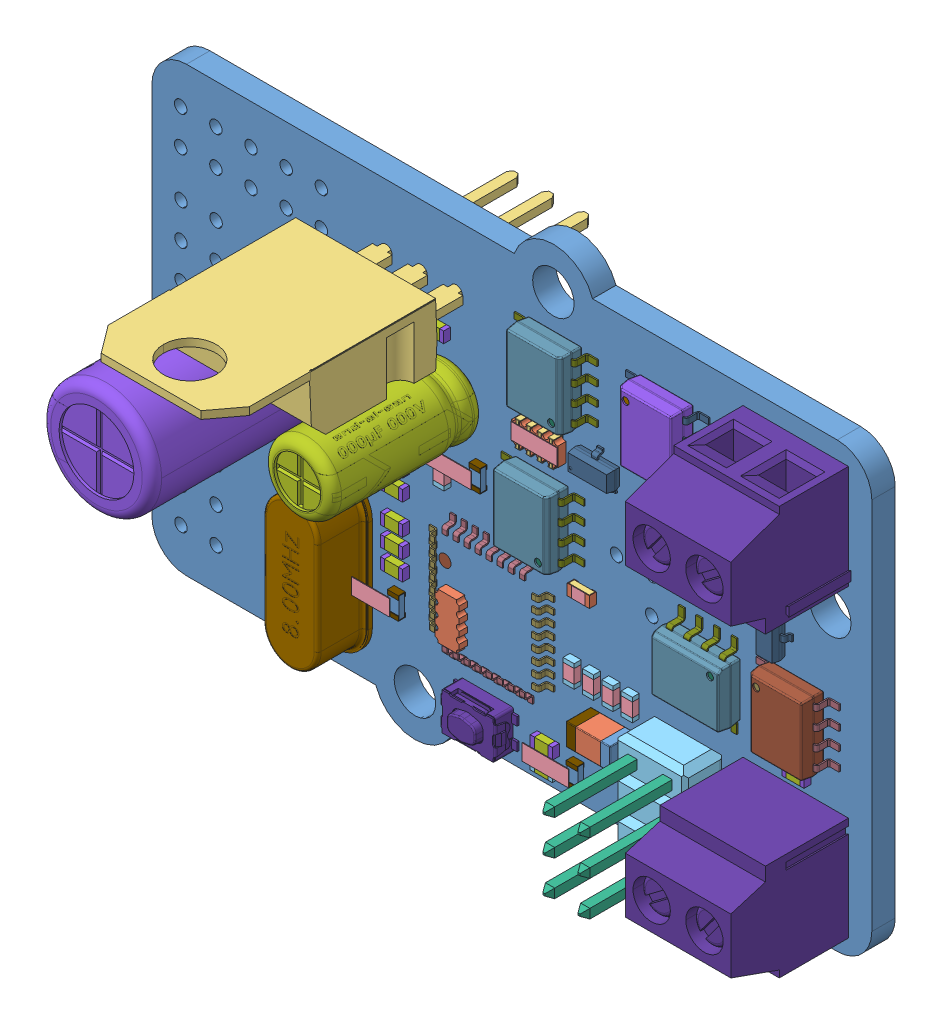
SolidWorks assembly DMotor_Rev1, configuration По умолчанию. Lengths in mm.
Overall size (52 36 28.9).
344 component instances, 44 part files, 0 mates.
Components (placement in the parent):
- DMotor_Rev1.step-1: DMotor_Rev1.step [По умолчанию] at origin size (52 36 28.9)
  - Board.step-1: Board.step [По умолчанию] at origin size (52 36 1.69)
    - Open CASCADE STEP translator 6.8 1.1.1.step-1: Open CASCADE STEP translator 6.8 1.1.1.step [По умолчанию] at (0 0 -1.692) size (52 36 1.69)
  - RN1.step-1: RN1.step [По умолчанию] at origin size (3.35 1.85 0.7)
    - 5778449216.step-1: 5778449216.step [По умолчанию] at (28.3 21.5 0) x (0 1 0) z (0 0 1) size (1.85 3.35 0.7)
      - body.step-1: body.step [По умолчанию] at (-0.875 -1.675 0) size (1.75 3.35 0.6)
        - Open_CASCADE_STEP_translator_6.8_25.1.1.step-1: Open_CASCADE_STEP_translator_6.8_25.1.1.step [По умолчанию] at origin size (1.75 3.35 0.6)
      - Mid_Pin.step-1: Mid_Pin.step [По умолчанию] at (-0.875 -1.2 0) size (0.3 0.38 0.7)
        - Open_CASCADE_STEP_translator_6.8_25.3.1.step-1: Open_CASCADE_STEP_translator_6.8_25.3.1.step [По умолчанию] at origin size (0.3 0.38 0.7)
      - Mid_Pin.step-2: Mid_Pin.step [По умолчанию] at (0.875 1.2 0) x (-1 0 0) z (0 0 1) size (0.3 0.38 0.7)
        - Open_CASCADE_STEP_translator_6.8_25.3.1.step-1: Open_CASCADE_STEP_translator_6.8_25.3.1.step [По умолчанию] at origin size (0.3 0.38 0.7)
      - Mid_Pin.step-3: Mid_Pin.step [По умолчанию] at (-0.875 -0.4 0) size (0.3 0.38 0.7)
        - Open_CASCADE_STEP_translator_6.8_25.3.1.step-1: Open_CASCADE_STEP_translator_6.8_25.3.1.step [По умолчанию] at origin size (0.3 0.38 0.7)
      - Mid_Pin.step-4: Mid_Pin.step [По умолчанию] at (0.875 0.4 0) x (-1 0 0) z (0 0 1) size (0.3 0.38 0.7)
        - Open_CASCADE_STEP_translator_6.8_25.3.1.step-1: Open_CASCADE_STEP_translator_6.8_25.3.1.step [По умолчанию] at origin size (0.3 0.38 0.7)
      - Mid_Pin.step-5: Mid_Pin.step [По умолчанию] at (-0.875 0.4 0) size (0.3 0.38 0.7)
        - Open_CASCADE_STEP_translator_6.8_25.3.1.step-1: Open_CASCADE_STEP_translator_6.8_25.3.1.step [По умолчанию] at origin size (0.3 0.38 0.7)
      - Mid_Pin.step-6: Mid_Pin.step [По умолчанию] at (0.875 -0.4 0) x (-1 0 0) z (0 0 1) size (0.3 0.38 0.7)
        - Open_CASCADE_STEP_translator_6.8_25.3.1.step-1: Open_CASCADE_STEP_translator_6.8_25.3.1.step [По умолчанию] at origin size (0.3 0.38 0.7)
      - Mid_Pin.step-7: Mid_Pin.step [По умолчанию] at (-0.875 1.2 0) size (0.3 0.38 0.7)
        - Open_CASCADE_STEP_translator_6.8_25.3.1.step-1: Open_CASCADE_STEP_translator_6.8_25.3.1.step [По умолчанию] at origin size (0.3 0.38 0.7)
      - Mid_Pin.step-8: Mid_Pin.step [По умолчанию] at (0.875 -1.2 0) x (-1 0 0) z (0 0 1) size (0.3 0.38 0.7)
        - Open_CASCADE_STEP_translator_6.8_25.3.1.step-1: Open_CASCADE_STEP_translator_6.8_25.3.1.step [По умолчанию] at origin size (0.3 0.38 0.7)
      - mark.step-1: mark.step [По умолчанию] at (-0.875 -1.675 0) size (1.15 3.35 0.05)
  - ICSP.step-1: ICSP.step [По умолчанию] at origin size (5.08 7.62 12.7)
    - 2x3_TH_Pitch_2_54mm.step-1: 2x3_TH_Pitch_2_54mm.step [По умолчанию] at (38.7601 0.89 0) x (0 1 0) z (1 0 0) size (7.62 12.7 5.08)
      - header2x3.step-1: header2x3.step [По умолчанию] at (0 1.4 0) size (7.62 2.8 5.08)
      - pin.step-1: pin.step [По умолчанию] at (1.29 -3.5 1.29) size (0.67 12.7 0.67)
      - pin.step-2: pin.step [По умолчанию] at (1.29 -3.5 -1.25) size (0.67 12.7 0.67)
      - pin.step-3: pin.step [По умолчанию] at (3.83 -3.5 1.29) size (0.67 12.7 0.67)
      - pin.step-4: pin.step [По умолчанию] at (3.83 -3.5 -1.25) size (0.67 12.7 0.67)
      - pin.step-5: pin.step [По умолчанию] at (6.37 -3.5 1.29) size (0.67 12.7 0.67)
      - pin.step-6: pin.step [По умолчанию] at (6.37 -3.5 -1.25) size (0.67 12.7 0.67)
  - C9.step-1: C9.step [По умолчанию] at origin size (1.6 0.8 0.5)
    - 5928350752.step-1: 5928350752.step [По умолчанию] at (17.8 11.1 0) size (1 0.8 0.5)
      - Extruded.step-1: Extruded.step [По умолчанию] at origin size (1 0.8 0.5)
    - 5928351312.step-1: 5928351312.step [По умолчанию] at (18.45 11.1 0) size (0.3 0.8 0.5)
      - Extruded-0.step-1: Extruded-0.step [По умолчанию] at origin size (0.3 0.8 0.5)
    - 5928351312.step-2: 5928351312.step [По умолчанию] at (17.15 11.1 0) size (0.3 0.8 0.5)
      - Extruded-0.step-1: Extruded-0.step [По умолчанию] at origin size (0.3 0.8 0.5)
  - C11.step-1: C11.step [По умолчанию] at origin size (1.6 0.8 0.5)
    - 5928350752.step-1: 5928350752.step [По умолчанию] at (17.8 8.3 0) size (1 0.8 0.5)
      - Extruded.step-1: Extruded.step [По умолчанию] at origin size (1 0.8 0.5)
    - 5928351312.step-1: 5928351312.step [По умолчанию] at (18.45 8.3 0) size (0.3 0.8 0.5)
      - Extruded-0.step-1: Extruded-0.step [По умолчанию] at origin size (0.3 0.8 0.5)
    - 5928351312.step-2: 5928351312.step [По умолчанию] at (17.15 8.3 0) size (0.3 0.8 0.5)
      - Extruded-0.step-1: Extruded-0.step [По умолчанию] at origin size (0.3 0.8 0.5)
  - Y1.step-1: Y1.step [По умолчанию] at origin size (4.65 11.35 5.59)
    - HC-49S.step-1: HC-49S.step [По умолчанию] at (13.6 6.8251 0) x (0 1 0) z (1 0 0) size (11.35 5.59 4.65)
  - VT2.step-1: VT2.step [По умолчанию] at origin size (2.9 2.3 1)
    - SOT23-3.step-1: SOT23-3.step [По умолчанию] at (31 21.9 0) x (1 0 0) z (0 -1 0) size (2.9 1 2.3)
  - VT1.step-1: VT1.step [По умолчанию] at origin size (2.3 2.9 1)
    - SOT23-3.step-1: SOT23-3.step [По умолчанию] at (45.2 19.5 0) x (0 -1 0) z (-1 0 0) size (2.9 1 2.3)
  - U1.step-1: U1.step [По умолчанию] at origin size (9 9 1.11)
    - 5778452896.step-1: 5778452896.step [По умолчанию] at (24.6 9.05 0) size (9 9 1.11)
      - body.step-1: body.step [По умолчанию] at (-3.5 -3.5 0) size (1.75 3.35 0.6)
        - Open_CASCADE_STEP_translator_6.8_25.1.1.step-1: Open_CASCADE_STEP_translator_6.8_25.1.1.step [По умолчанию] at origin size (1.75 3.35 0.6)
      - Open_CASCADE_STEP_translator_6.8_22.1.step-1: Open_CASCADE_STEP_translator_6.8_22.1.step [По умолчанию] at (-3.5 -3.5 0.001) size (0.89 0.89 0.01)
      - Leader.step-1: Leader.step [По умолчанию] at (-3.5 -2.8 0) x (-1 0 0) z (0 0 1) size (1 0.38 0.68)
      - Leader.step-2: Leader.step [По умолчанию] at (-3.5 -2 0) x (-1 0 0) z (0 0 1) size (1 0.38 0.68)
      - Leader.step-3: Leader.step [По умолчанию] at (-3.5 -1.2 0) x (-1 0 0) z (0 0 1) size (1 0.38 0.68)
      - Leader.step-4: Leader.step [По умолчанию] at (-3.5 -0.4 0) x (-1 0 0) z (0 0 1) size (1 0.38 0.68)
      - Leader.step-5: Leader.step [По умолчанию] at (-3.5 0.4 0) x (-1 0 0) z (0 0 1) size (1 0.38 0.68)
      - Leader.step-6: Leader.step [По умолчанию] at (-3.5 1.2 0) x (-1 0 0) z (0 0 1) size (1 0.38 0.68)
      - Leader.step-7: Leader.step [По умолчанию] at (-3.5 2 0) x (-1 0 0) z (0 0 1) size (1 0.38 0.68)
      - Leader.step-8: Leader.step [По умолчанию] at (-3.5 2.8 0) x (-1 0 0) z (0 0 1) size (1 0.38 0.68)
      - Leader.step-9: Leader.step [По умолчанию] at (3.5 -2.8 0) size (1 0.38 0.68)
      - Leader.step-10: Leader.step [По умолчанию] at (3.5 -2 0) size (1 0.38 0.68)
      - Leader.step-11: Leader.step [По умолчанию] at (3.5 -1.2 0) size (1 0.38 0.68)
      - Leader.step-12: Leader.step [По умолчанию] at (3.5 -0.4 0) size (1 0.38 0.68)
      - Leader.step-13: Leader.step [По умолчанию] at (3.5 0.4 0) size (1 0.38 0.68)
      - Leader.step-14: Leader.step [По умолчанию] at (3.5 1.2 0) size (1 0.38 0.68)
      - Leader.step-15: Leader.step [По умолчанию] at (3.5 2 0) size (1 0.38 0.68)
      - Leader.step-16: Leader.step [По умолчанию] at (3.5 2.8 0) size (1 0.38 0.68)
      - Leader-1.step-1: Leader-1.step [По умолчанию] at (-2.8 -3.5 0) x (0 -1 0) z (0 0 1) size (1 0.38 0.68)
      - Leader-1.step-2: Leader-1.step [По умолчанию] at (-2 -3.5 0) x (0 -1 0) z (0 0 1) size (1 0.38 0.68)
      - Leader-1.step-3: Leader-1.step [По умолчанию] at (-1.2 -3.5 0) x (0 -1 0) z (0 0 1) size (1 0.38 0.68)
      - Leader-1.step-4: Leader-1.step [По умолчанию] at (-0.4 -3.5 0) x (0 -1 0) z (0 0 1) size (1 0.38 0.68)
      - Leader-1.step-5: Leader-1.step [По умолчанию] at (0.4 -3.5 0) x (0 -1 0) z (0 0 1) size (1 0.38 0.68)
      - Leader-1.step-6: Leader-1.step [По умолчанию] at (1.2 -3.5 0) x (0 -1 0) z (0 0 1) size (1 0.38 0.68)
      - Leader-1.step-7: Leader-1.step [По умолчанию] at (2 -3.5 0) x (0 -1 0) z (0 0 1) size (1 0.38 0.68)
      - Leader-1.step-8: Leader-1.step [По умолчанию] at (2.8 -3.5 0) x (0 -1 0) z (0 0 1) size (1 0.38 0.68)
      - Leader-1.step-9: Leader-1.step [По умолчанию] at (-2.8 3.5 0) x (0 1 0) z (0 0 1) size (1 0.38 0.68)
      - Leader-1.step-10: Leader-1.step [По умолчанию] at (-2 3.5 0) x (0 1 0) z (0 0 1) size (1 0.38 0.68)
      - Leader-1.step-11: Leader-1.step [По умолчанию] at (-1.2 3.5 0) x (0 1 0) z (0 0 1) size (1 0.38 0.68)
      - Leader-1.step-12: Leader-1.step [По умолчанию] at (-0.4 3.5 0) x (0 1 0) z (0 0 1) size (1 0.38 0.68)
      - Leader-1.step-13: Leader-1.step [По умолчанию] at (0.4 3.5 0) x (0 1 0) z (0 0 1) size (1 0.38 0.68)
      - Leader-1.step-14: Leader-1.step [По умолчанию] at (1.2 3.5 0) x (0 1 0) z (0 0 1) size (1 0.38 0.68)
      - Leader-1.step-15: Leader-1.step [По умолчанию] at (2 3.5 0) x (0 1 0) z (0 0 1) size (1 0.38 0.68)
      - Leader-1.step-16: Leader-1.step [По умолчанию] at (2.8 3.5 0) x (0 1 0) z (0 0 1) size (1 0.38 0.68)
  - U2.step-1: U2.step [По умолчанию] at origin size (6 5.01 1.75)
    - 5778448736.step-1: 5778448736.step [По умолчанию] at (28.3 17.1 0) x (-1 0 0) z (0 0 1) size (6 5 1.75)
      - Body-1.step-1: Body-1.step [По умолчанию] at (-2 -2.5 0) size (4 5 1.65)
        - Open_CASCADE_STEP_translator_6.8_4.2.1.step-1: Open_CASCADE_STEP_translator_6.8_4.2.1.step [По умолчанию] at origin size (4 5 1.65)
      - Open_CASCADE_STEP_translator_6.8_4.1.step-1: Open_CASCADE_STEP_translator_6.8_4.1.step [По умолчанию] at (-2 -2.5 0.001) size (0.51 0.51 0.01)
      - Leader-2.step-1: Leader-2.step [По умолчанию] at (-2 -1.905 0) x (-1 0 0) z (0 0 1) size (1 0.42 0.97)
      - Leader-2.step-2: Leader-2.step [По умолчанию] at (-2 -0.635 0) x (-1 0 0) z (0 0 1) size (1 0.42 0.97)
      - Leader-2.step-3: Leader-2.step [По умолчанию] at (-2 0.635 0) x (-1 0 0) z (0 0 1) size (1 0.42 0.97)
      - Leader-2.step-4: Leader-2.step [По умолчанию] at (-2 1.905 0) x (-1 0 0) z (0 0 1) size (1 0.42 0.97)
      - Leader-2.step-5: Leader-2.step [По умолчанию] at (2 -1.905 0) size (1 0.42 0.97)
      - Leader-2.step-6: Leader-2.step [По умолчанию] at (2 -0.635 0) size (1 0.42 0.97)
      - Leader-2.step-7: Leader-2.step [По умолчанию] at (2 0.635 0) size (1 0.42 0.97)
      - Leader-2.step-8: Leader-2.step [По умолчанию] at (2 1.905 0) size (1 0.42 0.97)
  - RESET.step-1: RESET.step [По умолчанию] at origin size (4.6 2.8 1.94)
    - KMR221GLFS.step-1: KMR221GLFS.step [По умолчанию] at (24.2249 2.1749 0) x (-1 0 0) z (0 1 0) size (4.6 1.94 2.8)
  - R7.step-1: R7.step [По умолчанию] at origin size (3.35 1.75 1.15)
    - 5778454576.step-1: 5778454576.step [По умолчанию] at (23.8 17 0) x (0 1 0) z (0 0 1) size (1.75 3.35 1.15)
      - Terminal.step-1: Terminal.step [По умолчанию] at (-0.8 -0.4 0) size (0.3 0.8 0.5)
        - Open_CASCADE_STEP_translator_6.8_7.2.1.step-1: Open_CASCADE_STEP_translator_6.8_7.2.1.step [По умолчанию] at origin size (0.3 0.8 0.5)
      - Terminal.step-2: Terminal.step [По умолчанию] at (0.8 0.4 0) x (-1 0 0) z (0 0 1) size (0.3 0.8 0.5)
        - Open_CASCADE_STEP_translator_6.8_7.2.1.step-1: Open_CASCADE_STEP_translator_6.8_7.2.1.step [По умолчанию] at origin size (0.3 0.8 0.5)
      - Mid_Body.step-1: Mid_Body.step [По умолчанию] at (-0.8 -0.4 0) size (1.5 0.8 0.4)
      - mark.step-1: mark.step [По умолчанию] at (-0.5 -0.4 0.45) size (1.15 3.35 0.05)
  - R6.step-1: R6.step [По умолчанию] at origin size (1.6 0.8 0.5)
    - 5778452416.step-1: 5778452416.step [По умолчанию] at (31.3 13.4 0) x (1 0 0) z (0 0 1) size (1.6 0.8 0.5)
      - Terminal-1.step-1: Terminal-1.step [По умолчанию] at (-0.8 -0.4 0) size (0.3 0.8 0.5)
        - Open_CASCADE_STEP_translator_6.8_7.2.1-3.step-1: Open_CASCADE_STEP_translator_6.8_7.2.1-3.step [По умолчанию] at origin size (0.3 0.8 0.5)
      - Terminal-1.step-2: Terminal-1.step [По умолчанию] at (0.8 0.4 0) x (-1 0 0) z (0 0 1) size (0.3 0.8 0.5)
        - Open_CASCADE_STEP_translator_6.8_7.2.1-3.step-1: Open_CASCADE_STEP_translator_6.8_7.2.1-3.step [По умолчанию] at origin size (0.3 0.8 0.5)
      - Mid_Body-4.step-1: Mid_Body-4.step [По умолчанию] at (-0.8 -0.4 0) size (1.5 0.8 0.4)
      - Mark-5.step-1: Mark-5.step [По умолчанию] at (-0.5 -0.4 0.45) size (1 0.8 0.05)
  - R5.step-1: R5.step [По умолчанию] at origin size (1.6 0.8 0.5)
    - 5778448016.step-1: 5778448016.step [По умолчанию] at (28.625 1.175 0) x (-1 0 0) z (0 0 1) size (1.6 0.8 0.5)
      - Terminal-2.step-1: Terminal-2.step [По умолчанию] at (-0.8 -0.4 0) size (0.3 0.8 0.5)
        - Open_CASCADE_STEP_translator_6.8_7.2.1-6.step-1: Open_CASCADE_STEP_translator_6.8_7.2.1-6.step [По умолчанию] at origin size (0.3 0.8 0.5)
      - Terminal-2.step-2: Terminal-2.step [По умолчанию] at (0.8 0.4 0) x (-1 0 0) z (0 0 1) size (0.3 0.8 0.5)
        - Open_CASCADE_STEP_translator_6.8_7.2.1-6.step-1: Open_CASCADE_STEP_translator_6.8_7.2.1-6.step [По умолчанию] at origin size (0.3 0.8 0.5)
      - Mid_Body-7.step-1: Mid_Body-7.step [По умолчанию] at (-0.8 -0.4 0) size (1.5 0.8 0.4)
      - Mark-8.step-1: Mark-8.step [По умолчанию] at (-0.5 -0.4 0.45) size (1 0.8 0.05)
  - R4.step-1: R4.step [По умолчанию] at origin size (3.35 1.75 1.15)
    - 5778454576.step-1: 5778454576.step [По умолчанию] at (30.825 1.875 0) x (0 1 0) z (0 0 1) size (1.75 3.35 1.15)
      - Terminal.step-1: Terminal.step [По умолчанию] at (-0.8 -0.4 0) size (0.3 0.8 0.5)
        - Open_CASCADE_STEP_translator_6.8_7.2.1.step-1: Open_CASCADE_STEP_translator_6.8_7.2.1.step [По умолчанию] at origin size (0.3 0.8 0.5)
      - Terminal.step-2: Terminal.step [По умолчанию] at (0.8 0.4 0) x (-1 0 0) z (0 0 1) size (0.3 0.8 0.5)
        - Open_CASCADE_STEP_translator_6.8_7.2.1.step-1: Open_CASCADE_STEP_translator_6.8_7.2.1.step [По умолчанию] at origin size (0.3 0.8 0.5)
      - Mid_Body.step-1: Mid_Body.step [По умолчанию] at (-0.8 -0.4 0) size (1.5 0.8 0.4)
      - mark.step-1: mark.step [По умолчанию] at (-0.5 -0.4 0.45) size (1.15 3.35 0.05)
  - R2.step-1: R2.step [По умолчанию] at origin size (3.35 1.75 1.15)
    - 5778454576.step-1: 5778454576.step [По умолчанию] at (10.025 13.8 0) x (0 1 0) z (0 0 1) size (1.75 3.35 1.15)
      - Terminal.step-1: Terminal.step [По умолчанию] at (-0.8 -0.4 0) size (0.3 0.8 0.5)
        - Open_CASCADE_STEP_translator_6.8_7.2.1.step-1: Open_CASCADE_STEP_translator_6.8_7.2.1.step [По умолчанию] at origin size (0.3 0.8 0.5)
      - Terminal.step-2: Terminal.step [По умолчанию] at (0.8 0.4 0) x (-1 0 0) z (0 0 1) size (0.3 0.8 0.5)
        - Open_CASCADE_STEP_translator_6.8_7.2.1.step-1: Open_CASCADE_STEP_translator_6.8_7.2.1.step [По умолчанию] at origin size (0.3 0.8 0.5)
      - Mid_Body.step-1: Mid_Body.step [По умолчанию] at (-0.8 -0.4 0) size (1.5 0.8 0.4)
      - mark.step-1: mark.step [По умолчанию] at (-0.5 -0.4 0.45) size (1.15 3.35 0.05)
  - R3.step-1: R3.step [По умолчанию] at origin size (3.35 1.75 1.15)
    - 5778454576.step-1: 5778454576.step [По умолчанию] at (17.9 6.1 0) x (0 1 0) z (0 0 1) size (1.75 3.35 1.15)
      - Terminal.step-1: Terminal.step [По умолчанию] at (-0.8 -0.4 0) size (0.3 0.8 0.5)
        - Open_CASCADE_STEP_translator_6.8_7.2.1.step-1: Open_CASCADE_STEP_translator_6.8_7.2.1.step [По умолчанию] at origin size (0.3 0.8 0.5)
      - Terminal.step-2: Terminal.step [По умолчанию] at (0.8 0.4 0) x (-1 0 0) z (0 0 1) size (0.3 0.8 0.5)
        - Open_CASCADE_STEP_translator_6.8_7.2.1.step-1: Open_CASCADE_STEP_translator_6.8_7.2.1.step [По умолчанию] at origin size (0.3 0.8 0.5)
      - Mid_Body.step-1: Mid_Body.step [По умолчанию] at (-0.8 -0.4 0) size (1.5 0.8 0.4)
      - mark.step-1: mark.step [По умолчанию] at (-0.5 -0.4 0.45) size (1.15 3.35 0.05)
  - R1.step-1: R1.step [По умолчанию] at origin size (3.35 1.75 1.15)
    - 5778454576.step-1: 5778454576.step [По умолчанию] at (11.425 13.8 0) x (0 1 0) z (0 0 1) size (1.75 3.35 1.15)
      - Terminal.step-1: Terminal.step [По умолчанию] at (-0.8 -0.4 0) size (0.3 0.8 0.5)
        - Open_CASCADE_STEP_translator_6.8_7.2.1.step-1: Open_CASCADE_STEP_translator_6.8_7.2.1.step [По умолчанию] at origin size (0.3 0.8 0.5)
      - Terminal.step-2: Terminal.step [По умолчанию] at (0.8 0.4 0) x (-1 0 0) z (0 0 1) size (0.3 0.8 0.5)
        - Open_CASCADE_STEP_translator_6.8_7.2.1.step-1: Open_CASCADE_STEP_translator_6.8_7.2.1.step [По умолчанию] at origin size (0.3 0.8 0.5)
      - Mid_Body.step-1: Mid_Body.step [По умолчанию] at (-0.8 -0.4 0) size (1.5 0.8 0.4)
      - mark.step-1: mark.step [По умолчанию] at (-0.5 -0.4 0.45) size (1.15 3.35 0.05)
  - Q4.step-1: Q4.step [По умолчанию] at origin size (6 5 1.75)
    - 5778453696.step-1: 5778453696.step [По умолчанию] at (37.3 26.7 0) size (6 5 1.75)
      - Body-2.step-1: Body-2.step [По умолчанию] at (-2 -2.5 0) size (4 5 1.65)
        - Open_CASCADE_STEP_translator_6.8_4.2.1-9.step-1: Open_CASCADE_STEP_translator_6.8_4.2.1-9.step [По умолчанию] at origin size (4 5 1.65)
      - Open_CASCADE_STEP_translator_6.8_4.1-10.step-1: Open_CASCADE_STEP_translator_6.8_4.1-10.step [По умолчанию] at (-2 -2.5 0.001) size (0.51 0.51 0.01)
      - Leader-11.step-1: Leader-11.step [По умолчанию] at (-2 -1.905 0) x (-1 0 0) z (0 0 1) size (1 0.42 0.97)
      - Leader-11.step-2: Leader-11.step [По умолчанию] at (-2 -0.635 0) x (-1 0 0) z (0 0 1) size (1 0.42 0.97)
      - Leader-11.step-3: Leader-11.step [По умолчанию] at (-2 0.635 0) x (-1 0 0) z (0 0 1) size (1 0.42 0.97)
      - Leader-11.step-4: Leader-11.step [По умолчанию] at (-2 1.905 0) x (-1 0 0) z (0 0 1) size (1 0.42 0.97)
      - Leader-11.step-5: Leader-11.step [По умолчанию] at (2 -1.905 0) size (1 0.42 0.97)
      - Leader-11.step-6: Leader-11.step [По умолчанию] at (2 -0.635 0) size (1 0.42 0.97)
      - Leader-11.step-7: Leader-11.step [По умолчанию] at (2 0.635 0) size (1 0.42 0.97)
      - Leader-11.step-8: Leader-11.step [По умолчанию] at (2 1.905 0) size (1 0.42 0.97)
  - Q3.step-1: Q3.step [По умолчанию] at origin size (6 5.01 1.75)
    - 5778448736.step-1: 5778448736.step [По умолчанию] at (29.25 26.3 0) x (-1 0 0) z (0 0 1) size (6 5 1.75)
      - Body-1.step-1: Body-1.step [По умолчанию] at (-2 -2.5 0) size (4 5 1.65)
        - Open_CASCADE_STEP_translator_6.8_4.2.1.step-1: Open_CASCADE_STEP_translator_6.8_4.2.1.step [По умолчанию] at origin size (4 5 1.65)
      - Open_CASCADE_STEP_translator_6.8_4.1.step-1: Open_CASCADE_STEP_translator_6.8_4.1.step [По умолчанию] at (-2 -2.5 0.001) size (0.51 0.51 0.01)
      - Leader-2.step-1: Leader-2.step [По умолчанию] at (-2 -1.905 0) x (-1 0 0) z (0 0 1) size (1 0.42 0.97)
      - Leader-2.step-2: Leader-2.step [По умолчанию] at (-2 -0.635 0) x (-1 0 0) z (0 0 1) size (1 0.42 0.97)
      - Leader-2.step-3: Leader-2.step [По умолчанию] at (-2 0.635 0) x (-1 0 0) z (0 0 1) size (1 0.42 0.97)
      - Leader-2.step-4: Leader-2.step [По умолчанию] at (-2 1.905 0) x (-1 0 0) z (0 0 1) size (1 0.42 0.97)
      - Leader-2.step-5: Leader-2.step [По умолчанию] at (2 -1.905 0) size (1 0.42 0.97)
      - Leader-2.step-6: Leader-2.step [По умолчанию] at (2 -0.635 0) size (1 0.42 0.97)
      - Leader-2.step-7: Leader-2.step [По умолчанию] at (2 0.635 0) size (1 0.42 0.97)
      - Leader-2.step-8: Leader-2.step [По умолчанию] at (2 1.905 0) size (1 0.42 0.97)
  - Q2.step-1: Q2.step [По умолчанию] at origin size (6 5.01 1.75)
    - 5778447616.step-1: 5778447616.step [По умолчанию] at (46.725 13.495 0) x (1 0 0) z (0 0 1) size (6 5 1.75)
      - Body-3.step-1: Body-3.step [По умолчанию] at (-2 -2.5 0) size (4 5 1.65)
        - Open_CASCADE_STEP_translator_6.8_4.2.1-12.step-1: Open_CASCADE_STEP_translator_6.8_4.2.1-12.step [По умолчанию] at origin size (4 5 1.65)
      - Open_CASCADE_STEP_translator_6.8_4.1-13.step-1: Open_CASCADE_STEP_translator_6.8_4.1-13.step [По умолчанию] at (-2 -2.5 0.001) size (0.51 0.51 0.01)
      - Leader-14.step-1: Leader-14.step [По умолчанию] at (-2 -1.905 0) x (-1 0 0) z (0 0 1) size (1 0.42 0.97)
      - Leader-14.step-2: Leader-14.step [По умолчанию] at (-2 -0.635 0) x (-1 0 0) z (0 0 1) size (1 0.42 0.97)
      - Leader-14.step-3: Leader-14.step [По умолчанию] at (-2 0.635 0) x (-1 0 0) z (0 0 1) size (1 0.42 0.97)
      - Leader-14.step-4: Leader-14.step [По умолчанию] at (-2 1.905 0) x (-1 0 0) z (0 0 1) size (1 0.42 0.97)
      - Leader-14.step-5: Leader-14.step [По умолчанию] at (2 -1.905 0) size (1 0.42 0.97)
      - Leader-14.step-6: Leader-14.step [По умолчанию] at (2 -0.635 0) size (1 0.42 0.97)
      - Leader-14.step-7: Leader-14.step [По умолчанию] at (2 0.635 0) size (1 0.42 0.97)
      - Leader-14.step-8: Leader-14.step [По умолчанию] at (2 1.905 0) size (1 0.42 0.97)
  - Q1.step-1: Q1.step [По умолчанию] at origin size (5.01 6 1.75)
    - 5778450736.step-1: 5778450736.step [По умолчанию] at (40.225 13.0265 0) x (0 -1 0) z (0 0 1) size (6 5 1.75)
      - Body-4.step-1: Body-4.step [По умолчанию] at (-2 -2.5 0) size (4 5 1.65)
        - Open_CASCADE_STEP_translator_6.8_4.2.1-15.step-1: Open_CASCADE_STEP_translator_6.8_4.2.1-15.step [По умолчанию] at origin size (4 5 1.65)
      - Open_CASCADE_STEP_translator_6.8_4.1-16.step-1: Open_CASCADE_STEP_translator_6.8_4.1-16.step [По умолчанию] at (-2 -2.5 0.001) size (0.51 0.51 0.01)
      - Leader-17.step-1: Leader-17.step [По умолчанию] at (-2 -1.905 0) x (-1 0 0) z (0 0 1) size (1 0.42 0.97)
      - Leader-17.step-2: Leader-17.step [По умолчанию] at (-2 -0.635 0) x (-1 0 0) z (0 0 1) size (1 0.42 0.97)
      - Leader-17.step-3: Leader-17.step [По умолчанию] at (-2 0.635 0) x (-1 0 0) z (0 0 1) size (1 0.42 0.97)
      - Leader-17.step-4: Leader-17.step [По умолчанию] at (-2 1.905 0) x (-1 0 0) z (0 0 1) size (1 0.42 0.97)
      - Leader-17.step-5: Leader-17.step [По умолчанию] at (2 -1.905 0) size (1 0.42 0.97)
      - Leader-17.step-6: Leader-17.step [По умолчанию] at (2 -0.635 0) size (1 0.42 0.97)
      - Leader-17.step-7: Leader-17.step [По умолчанию] at (2 0.635 0) size (1 0.42 0.97)
      - Leader-17.step-8: Leader-17.step [По умолчанию] at (2 1.905 0) size (1 0.42 0.97)
  - P3.step-1: P3.step [По умолчанию] at origin size (7.81 7.5 12)
    - KLS2-340-3.81.step-1: KLS2-340-3.81.step [По умолчанию] at (46.5051 27.0001 0) size (7.81 7.5 12)
  - P2.step-1: P2.step [По умолчанию] at origin size (7.81 7.5 12)
    - KLS2-340-3.81.step-1: KLS2-340-3.81.step [По умолчанию] at (46.5049 4.9999 0) x (-1 0 0) z (0 0 1) size (7.81 7.5 12)
  - L3.step-1: L3.step [По умолчанию] at origin size (3.2 1.6 1.8)
    - 5778447296.step-1: 5778447296.step [По умолчанию] at (33.3 5.6 0) x (1 0 0) z (0 0 1) size (3.2 1.6 1.8)
      - Terminal-3.step-1: Terminal-3.step [По умолчанию] at (-1.6 -0.8 0) size (3.2 1.6 1.8)
        - Open_CASCADE_STEP_translator_6.8_9.1.1.step-1: Open_CASCADE_STEP_translator_6.8_9.1.1.step [По умолчанию] at origin size (0.7 1.6 1.8)
        - Open_CASCADE_STEP_translator_6.8_9.1.2.step-1: Open_CASCADE_STEP_translator_6.8_9.1.2.step [По умолчанию] at origin size (0.7 1.6 1.8)
      - Mid_Body-18.step-1: Mid_Body-18.step [По умолчанию] at (-1.6 -0.8 0) size (1.8 1.6 1.8)
        - Open_CASCADE_STEP_translator_6.8_9.2.1.step-1: Open_CASCADE_STEP_translator_6.8_9.2.1.step [По умолчанию] at origin size (1.8 1.6 1.8)
  - DA1.step-1: DA1.step [По умолчанию] at origin size (10.2 4.5 28.9)
    - TO220.step-1: TO220.step [По умолчанию] at (19.4399 30.3489 4) x (1 0 0) z (0 -1 0) size (10.2 28.9 4.5)
  - C21.step-1: C21.step [По умолчанию] at origin size (0.8 1.6 0.5)
    - 5928349552.step-1: 5928349552.step [По умолчанию] at (41.7 26.9 0) size (0.8 1 0.5)
      - Extruded-19.step-1: Extruded-19.step [По умолчанию] at origin size (0.8 1 0.5)
    - 5928349232.step-1: 5928349232.step [По умолчанию] at (41.7 26.25 0) size (0.8 0.3 0.5)
      - Extruded-20.step-1: Extruded-20.step [По умолчанию] at origin size (0.8 0.3 0.5)
    - 5928349232.step-2: 5928349232.step [По умолчанию] at (41.7 27.55 0) size (0.8 0.3 0.5)
      - Extruded-20.step-1: Extruded-20.step [По умолчанию] at origin size (0.8 0.3 0.5)
  - C20.step-1: C20.step [По умолчанию] at origin size (1.6 0.8 0.5)
    - 5928351312.step-1: 5928351312.step [По умолчанию] at (46.15 9.9 0) size (0.3 0.8 0.5)
      - Extruded-0.step-1: Extruded-0.step [По умолчанию] at origin size (0.3 0.8 0.5)
    - 5928351312.step-2: 5928351312.step [По умолчанию] at (47.45 9.9 0) size (0.3 0.8 0.5)
      - Extruded-0.step-1: Extruded-0.step [По умолчанию] at origin size (0.3 0.8 0.5)
    - 5928350752.step-1: 5928350752.step [По умолчанию] at (46.8 9.9 0) size (1 0.8 0.5)
      - Extruded.step-1: Extruded.step [По умолчанию] at origin size (1 0.8 0.5)
  - C19.step-1: C19.step [По умолчанию] at origin size (0.8 1.6 0.5)
    - 5928349552.step-1: 5928349552.step [По умолчанию] at (21.2 15.9 0) size (0.8 1 0.5)
      - Extruded-19.step-1: Extruded-19.step [По умолчанию] at origin size (0.8 1 0.5)
    - 5928349232.step-1: 5928349232.step [По умолчанию] at (21.2 16.55 0) size (0.8 0.3 0.5)
      - Extruded-20.step-1: Extruded-20.step [По умолчанию] at origin size (0.8 0.3 0.5)
    - 5928349232.step-2: 5928349232.step [По умолчанию] at (21.2 15.25 0) size (0.8 0.3 0.5)
      - Extruded-20.step-1: Extruded-20.step [По умолчанию] at origin size (0.8 0.3 0.5)
  - C18.step-1: C18.step [По умолчанию] at origin size (1.6 0.8 0.5)
    - 5928351312.step-1: 5928351312.step [По умолчанию] at (27.975 2.575 0) size (0.3 0.8 0.5)
      - Extruded-0.step-1: Extruded-0.step [По умолчанию] at origin size (0.3 0.8 0.5)
    - 5928351312.step-2: 5928351312.step [По умолчанию] at (29.275 2.575 0) size (0.3 0.8 0.5)
      - Extruded-0.step-1: Extruded-0.step [По умолчанию] at origin size (0.3 0.8 0.5)
    - 5928350752.step-1: 5928350752.step [По умолчанию] at (28.625 2.575 0) size (1 0.8 0.5)
      - Extruded.step-1: Extruded.step [По умолчанию] at origin size (1 0.8 0.5)
  - C17.step-1: C17.step [По умолчанию] at origin size (0.8 1.6 0.5)
    - 5928349552.step-1: 5928349552.step [По умолчанию] at (10.3 5.2 0) size (0.8 1 0.5)
      - Extruded-19.step-1: Extruded-19.step [По умолчанию] at origin size (0.8 1 0.5)
    - 5928349232.step-1: 5928349232.step [По умолчанию] at (10.3 4.55 0) size (0.8 0.3 0.5)
      - Extruded-20.step-1: Extruded-20.step [По умолчанию] at origin size (0.8 0.3 0.5)
    - 5928349232.step-2: 5928349232.step [По умолчанию] at (10.3 5.85 0) size (0.8 0.3 0.5)
      - Extruded-20.step-1: Extruded-20.step [По умолчанию] at origin size (0.8 0.3 0.5)
  - C16.step-1: C16.step [По умолчанию] at origin size (0.8 1.6 0.5)
    - 5928349552.step-1: 5928349552.step [По умолчанию] at (10.3 8.2 0) size (0.8 1 0.5)
      - Extruded-19.step-1: Extruded-19.step [По умолчанию] at origin size (0.8 1 0.5)
    - 5928349232.step-1: 5928349232.step [По умолчанию] at (10.3 7.55 0) size (0.8 0.3 0.5)
      - Extruded-20.step-1: Extruded-20.step [По умолчанию] at origin size (0.8 0.3 0.5)
    - 5928349232.step-2: 5928349232.step [По умолчанию] at (10.3 8.85 0) size (0.8 0.3 0.5)
      - Extruded-20.step-1: Extruded-20.step [По умолчанию] at origin size (0.8 0.3 0.5)
  - C15.step-1: C15.step [По умолчанию] at origin size (0.8 1.6 0.5)
    - 5928349552.step-1: 5928349552.step [По умолчанию] at (30.6 8.2 0) size (0.8 1 0.5)
      - Extruded-19.step-1: Extruded-19.step [По умолчанию] at origin size (0.8 1 0.5)
    - 5928349232.step-1: 5928349232.step [По умолчанию] at (30.6 7.55 0) size (0.8 0.3 0.5)
      - Extruded-20.step-1: Extruded-20.step [По умолчанию] at origin size (0.8 0.3 0.5)
    - 5928349232.step-2: 5928349232.step [По умолчанию] at (30.6 8.85 0) size (0.8 0.3 0.5)
      - Extruded-20.step-1: Extruded-20.step [По умолчанию] at origin size (0.8 0.3 0.5)
  - C14.step-1: C14.step [По умолчанию] at origin size (0.8 1.6 0.5)
    - 5928349552.step-1: 5928349552.step [По умолчанию] at (32 8.2 0) size (0.8 1 0.5)
      - Extruded-19.step-1: Extruded-19.step [По умолчанию] at origin size (0.8 1 0.5)
    - 5928349232.step-1: 5928349232.step [По умолчанию] at (32 7.55 0) size (0.8 0.3 0.5)
      - Extruded-20.step-1: Extruded-20.step [По умолчанию] at origin size (0.8 0.3 0.5)
    - 5928349232.step-2: 5928349232.step [По умолчанию] at (32 8.85 0) size (0.8 0.3 0.5)
      - Extruded-20.step-1: Extruded-20.step [По умолчанию] at origin size (0.8 0.3 0.5)
  - C13.step-1: C13.step [По умолчанию] at origin size (0.8 1.6 0.5)
    - 5928349552.step-1: 5928349552.step [По умолчанию] at (33.4 8.2 0) size (0.8 1 0.5)
      - Extruded-19.step-1: Extruded-19.step [По умолчанию] at origin size (0.8 1 0.5)
    - 5928349232.step-1: 5928349232.step [По умолчанию] at (33.4 7.55 0) size (0.8 0.3 0.5)
      - Extruded-20.step-1: Extruded-20.step [По умолчанию] at origin size (0.8 0.3 0.5)
    - 5928349232.step-2: 5928349232.step [По умолчанию] at (33.4 8.85 0) size (0.8 0.3 0.5)
      - Extruded-20.step-1: Extruded-20.step [По умолчанию] at origin size (0.8 0.3 0.5)
  - C12.step-1: C12.step [По умолчанию] at origin size (0.8 1.6 0.5)
    - 5928349552.step-1: 5928349552.step [По умолчанию] at (34.8 8.2 0) size (0.8 1 0.5)
      - Extruded-19.step-1: Extruded-19.step [По умолчанию] at origin size (0.8 1 0.5)
    - 5928349232.step-1: 5928349232.step [По умолчанию] at (34.8 7.55 0) size (0.8 0.3 0.5)
      - Extruded-20.step-1: Extruded-20.step [По умолчанию] at origin size (0.8 0.3 0.5)
    - 5928349232.step-2: 5928349232.step [По умолчанию] at (34.8 8.85 0) size (0.8 0.3 0.5)
      - Extruded-20.step-1: Extruded-20.step [По умолчанию] at origin size (0.8 0.3 0.5)
  - C10.step-1: C10.step [По умолчанию] at origin size (1.6 0.8 0.5)
    - 5928350752.step-1: 5928350752.step [По умолчанию] at (17.8 9.7 0) size (1 0.8 0.5)
      - Extruded.step-1: Extruded.step [По умолчанию] at origin size (1 0.8 0.5)
    - 5928351312.step-1: 5928351312.step [По умолчанию] at (18.45 9.7 0) size (0.3 0.8 0.5)
      - Extruded-0.step-1: Extruded-0.step [По умолчанию] at origin size (0.3 0.8 0.5)
    - 5928351312.step-2: 5928351312.step [По умолчанию] at (17.15 9.7 0) size (0.3 0.8 0.5)
      - Extruded-0.step-1: Extruded-0.step [По умолчанию] at origin size (0.3 0.8 0.5)
  - C8.step-1: C8.step [По умолчанию] at origin size (1.6 0.8 0.5)
    - 5928350752.step-1: 5928350752.step [По умолчанию] at (17.8 13.3 0) size (1 0.8 0.5)
      - Extruded.step-1: Extruded.step [По умолчанию] at origin size (1 0.8 0.5)
    - 5928351312.step-1: 5928351312.step [По умолчанию] at (18.45 13.3 0) size (0.3 0.8 0.5)
      - Extruded-0.step-1: Extruded-0.step [По умолчанию] at origin size (0.3 0.8 0.5)
    - 5928351312.step-2: 5928351312.step [По умолчанию] at (17.15 13.3 0) size (0.3 0.8 0.5)
      - Extruded-0.step-1: Extruded-0.step [По умолчанию] at origin size (0.3 0.8 0.5)
  - C7.step-1: C7.step [По умолчанию] at origin size (1.6 0.8 0.5)
    - 5928350752.step-1: 5928350752.step [По умолчанию] at (17.8 14.8 0) size (1 0.8 0.5)
      - Extruded.step-1: Extruded.step [По умолчанию] at origin size (1 0.8 0.5)
    - 5928351312.step-1: 5928351312.step [По умолчанию] at (18.45 14.8 0) size (0.3 0.8 0.5)
      - Extruded-0.step-1: Extruded-0.step [По умолчанию] at origin size (0.3 0.8 0.5)
    - 5928351312.step-2: 5928351312.step [По умолчанию] at (17.15 14.8 0) size (0.3 0.8 0.5)
      - Extruded-0.step-1: Extruded-0.step [По умолчанию] at origin size (0.3 0.8 0.5)
  - C6.step-1: C6.step [По умолчанию] at origin size (3.7 2.93 2.03)
    - TANT-B.step-1: TANT-B.step [По умолчанию] at (17.8999 17.1999 0) x (-1 0 0) z (0 0 1) size (3.7 2.93 2.03)
  - C5.step-1: C5.step [По умолчанию] at origin size (5.05 5.02 13.81)
    - Cap-EL(5x11-2)T.step-1: Cap-EL(5x11-2)T.step [По умолчанию] at (21.8001 21.2001 0.3) x (1 0 0) z (0 0 1) size (5.05 5.02 13.81)
  - C4.step-1: C4.step [По умолчанию] at origin size (1.6 0.8 0.5)
    - 5928350752.step-1: 5928350752.step [По умолчанию] at (20.775 24.7 0) size (1 0.8 0.5)
      - Extruded.step-1: Extruded.step [По умолчанию] at origin size (1 0.8 0.5)
    - 5928351312.step-1: 5928351312.step [По умолчанию] at (21.425 24.7 0) size (0.3 0.8 0.5)
      - Extruded-0.step-1: Extruded-0.step [По умолчанию] at origin size (0.3 0.8 0.5)
    - 5928351312.step-2: 5928351312.step [По умолчанию] at (20.125 24.7 0) size (0.3 0.8 0.5)
      - Extruded-0.step-1: Extruded-0.step [По умолчанию] at origin size (0.3 0.8 0.5)
  - C3.step-1: C3.step [По умолчанию] at origin size (1.6 0.8 0.5)
    - 5928350752.step-1: 5928350752.step [По умолчанию] at (17.775 24.7 0) size (1 0.8 0.5)
      - Extruded.step-1: Extruded.step [По умолчанию] at origin size (1 0.8 0.5)
    - 5928351312.step-1: 5928351312.step [По умолчанию] at (17.125 24.7 0) size (0.3 0.8 0.5)
      - Extruded-0.step-1: Extruded-0.step [По умолчанию] at origin size (0.3 0.8 0.5)
    - 5928351312.step-2: 5928351312.step [По умолчанию] at (18.425 24.7 0) size (0.3 0.8 0.5)
      - Extruded-0.step-1: Extruded-0.step [По умолчанию] at origin size (0.3 0.8 0.5)
  - C2.step-1: C2.step [По умолчанию] at origin size (1.6 0.8 0.5)
    - 5928350752.step-1: 5928350752.step [По умолчанию] at (17.8 23.2 0) size (1 0.8 0.5)
      - Extruded.step-1: Extruded.step [По умолчанию] at origin size (1 0.8 0.5)
    - 5928351312.step-1: 5928351312.step [По умолчанию] at (17.15 23.2 0) size (0.3 0.8 0.5)
      - Extruded-0.step-1: Extruded-0.step [По умолчанию] at origin size (0.3 0.8 0.5)
    - 5928351312.step-2: 5928351312.step [По умолчанию] at (18.45 23.2 0) size (0.3 0.8 0.5)
      - Extruded-0.step-1: Extruded-0.step [По умолчанию] at origin size (0.3 0.8 0.5)
  - C1.step-1: C1.step [По умолчанию] at origin size (8.01 8 19.31)
    - Cap-EL(8x16-3_5).step-1: Cap-EL(8x16-3_5).step [По умолчанию] at (12.4999 21 0.5) x (-1 0 0) z (0 0 1) size (8.01 8 19.31)
